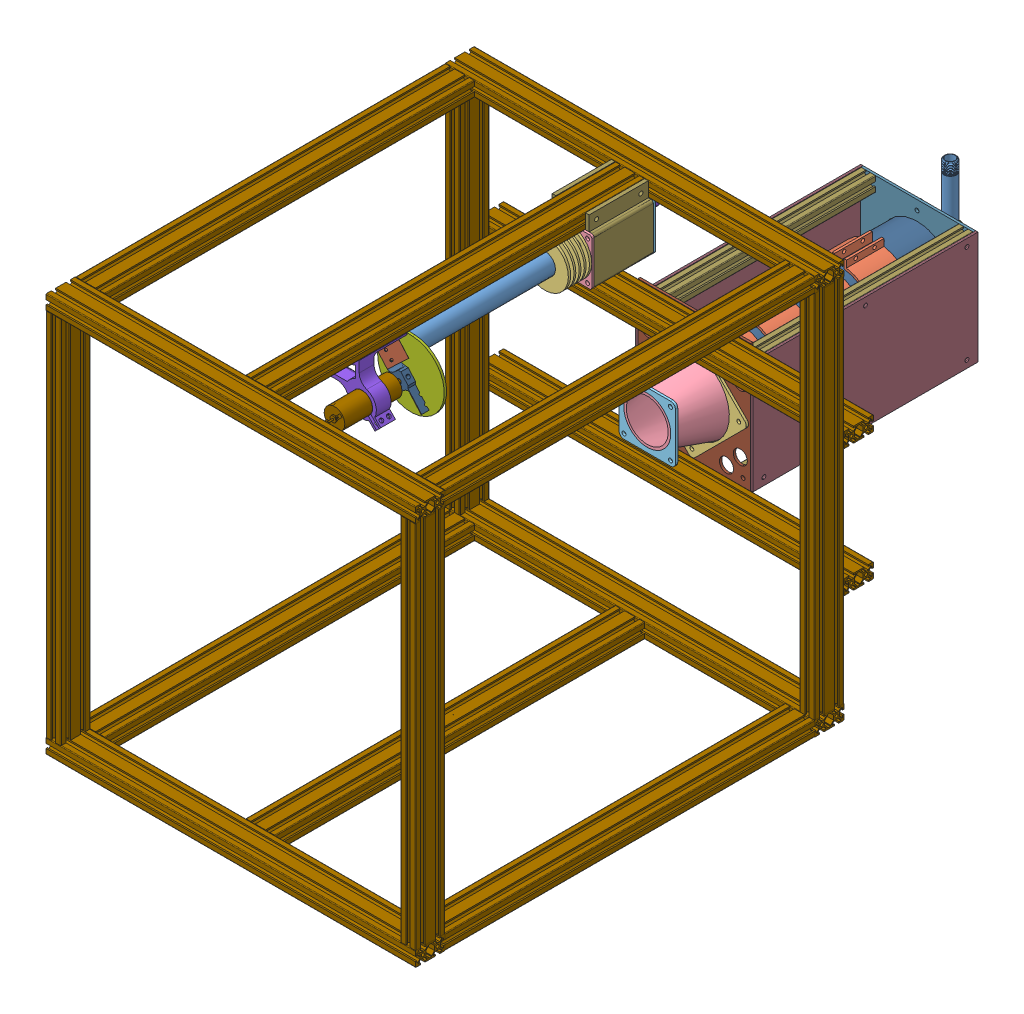
SolidWorks assembly extruder 1 assembly, configuration Default. Lengths in mm.
Overall size (500 540 979.81).
58 component instances, 30 part files, 85 mates.
Components (placement in the parent):
- extruder barrel_rev01-1: extruder barrel_rev01 [Default] at (188.8223 217.5446 43.8354) size (28.57 28.57 304.8)
- nozzle_rev01-1: nozzle_rev01 [Default] at (188.8223 217.5446 329.5854) size (28.57 28.57 31.75)
- barrel lock-1: barrel lock [Default] at (188.8223 217.5446 154.9604) x (-0.997738 -0.067218 0) z (0.067218 -0.997738 0) size (63.5 31.75 63.5)
- barrel lock mount-1: barrel lock mount [Default] at (188.8223 217.5446 120.0354) x (1 0 0) z (0 -1 0) size (63.5 3.17 63.5)
- thrust bearing plate-1: thrust bearing plate [Default] at (188.8223 217.5446 40.0354) x (1 0 0) z (0 1 0) size (63.5 3.17 63.5)
- 5909K310_THRUST NEEDLE-ROLLER BEARING-1: 5909K310_THRUST NEEDLE-ROLLER BEARING [5909K31] at (188.8223 217.5446 42.0304) x (1 0 0) z (0 -1 0) size (23.81 19.84 23.81)
- 5909K440_THRUST NEEDLE-ROLLER BEARING-1: 5909K440_THRUST NEEDLE-ROLLER BEARING [5909K44] at (188.8223 217.5446 41.0382) x (0 0 -1) z (0.082579 0.996584 0) size (0.81 23.81 23.81)
- 5909K440_THRUST NEEDLE-ROLLER BEARING-2: 5909K440_THRUST NEEDLE-ROLLER BEARING [5909K44] at (188.8223 217.5446 43.8354) x (0 0 -1) z (1 0 0) size (0.81 23.81 23.81)
- screw standin-1: screw standin [Default] at (188.8223 217.5446 310.5354) x (1 0 0) z (0 1 0) size (19.55 342.9 19.55)
- 500mm 2040-1: 500mm 2040 [Default] at (188.8223 259.2946 540.0354) x (0 -1 0) z (0 0 1) size (20 40 500)
- 500mm 2040-2: 500mm 2040 [Default] at (-61.3618 259.2946 560.0354) x (0 1 0) z (-1 0 0) size (20 40 500)
- 500mm 2040-3: 500mm 2040 [Default] at (-51.3618 249.2946 560.0354) x (1 0 0) z (0 1 0) size (20 40 500)
- 500mm 2040-4: 500mm 2040 [Default] at (428.6382 -250.7054 560.0354) x (1 0 0) z (0 -1 0) size (20 40 500)
- 500mm 2040-5: 500mm 2040 [Default] at (-61.3618 -260.7054 560.0354) x (0 1 0) z (-1 0 0) size (20 40 500)
- 500mm 2040-6: 500mm 2040 [Default] at (418.6382 259.2946 540.0354) x (0 1 0) z (0 0 1) size (20 40 500)
- 500mm 2040-7: 500mm 2040 [Default] at (-41.3618 259.2946 540.0354) x (0 1 0) z (0 0 1) size (20 40 500)
- 500mm 2040-8: 500mm 2040 [Default] at (418.6382 -260.7054 540.0354) x (0 1 0) z (0 0 1) size (20 40 500)
- 500mm 2040-9: 500mm 2040 [Default] at (-41.3618 -260.7054 540.0354) x (0 -1 0) z (0 0 1) size (20 40 500)
- 500mm 2040-10: 500mm 2040 [Default] at (-61.3618 -260.7054 20.0354) x (0 1 0) z (-1 0 0) size (20 40 500)
- 500mm 2040-11: 500mm 2040 [Default] at (-61.3618 259.2946 20.0354) x (0 -1 0) z (-1 0 0) size (20 40 500)
- 500mm 2040-12: 500mm 2040 [Default] at (-51.3618 249.2946 20.0354) x (-1 0 0) z (0 1 0) size (20 40 500)
- 500mm 2040-13: 500mm 2040 [Default] at (428.6382 249.2946 20.0354) x (1 0 0) z (0 1 0) size (20 40 500)
- 500mm 2040-14: 500mm 2040 [Default] at (188.8164 -260.7054 540.0354) x (0 -1 0) z (0 0 1) size (20 40 500)
- dryer stand alone-1: dryer stand alone [Default] at (381.6192 -132.2091 21.3365) x (0 1 0) z (-1 0 0) size (209.74 423.31 158.7)
  - tube-1: tube [Default] at (103.5422 61.3012 185.6839) size (164.34 304.8 101.6)
  - flange rev01-1: flange rev01 [Default] at (103.5422 61.3012 185.6839) x (-1 0 0) z (0 0 -1) size (192.4 3.17 152.4)
  - HFS5-2020-299-1: HFS5-2020-299 [Default] at (169.7422 63.9262 119.4839) x (-1 0 0) z (0 -1 0) size (20 20 298.45)
  - HFS5-2020-299-2: HFS5-2020-299 [Default] at (37.3422 63.9262 119.4839) x (-1 0 0) z (0 -1 0) size (20 20 298.45)
  - HFS5-2020-299-3: HFS5-2020-299 [Default] at (169.7422 63.9262 251.8839) x (-1 0 0) z (0 -1 0) size (20 20 298.45)
  - HFS5-2020-299-4: HFS5-2020-299 [Default] at (37.3422 363.4762 251.8839) x (-1 0 0) z (0 1 0) size (20 20 298.45)
  - side plate 1_16-1: side plate 1_16 [Default] at (103.5422 213.7012 263.4587) x (-1 0 0) z (0 0 -1) size (152.4 304.8 1.57)
  - side plate 1_16-2: side plate 1_16 [Default] at (103.5422 213.7012 265.0335) x (-1 0 0) z (0 0 -1) size (152.4 304.8 1.57)
  - flange rev02-1: flange rev02 [Default] at (103.5422 362.9262 185.6839) x (-1 0 0) z (0 0 -1) size (152.4 3.17 152.4)
  - top cover-1: top cover [Default] at (103.5422 369.2762 185.6839) x (-0.707107 0 -0.707107) z (0 -1 0) size (107.76 107.76 3.17)
  - 4452K413_TYPE 316 STAINLESS STL THREADED PIPE FITTING-2: 4452K413_TYPE 316 STAINLESS STL THREADED PIPE FITTING [4452K413] at (103.5422 407.8982 185.6839) x (-1 0 0) z (0 0 1) size (37.28 37.03 30.11)
  - 4548K159_STD-WALL TYPE 316-316L SS THRD PIPE NIPPLE-1: 4548K159_STD-WALL TYPE 316-316L SS THRD PIPE NIPPLE [4548K159] at (103.5422 292.6762 185.6839) x (0 1 0) z (0 0 1) size (203.35 17.91 17.78)
  - 4464K498_TYPE 304 STAINLESS STL THREADED PIPE FITTING-1: 4464K498_TYPE 304 STAINLESS STL THREADED PIPE FITTING [4464K498] at (103.5422 180.2482 185.6839) x (-0.837169 0 -0.546944) z (0 1 0) size (25.91 25.91 21.03)
  - 4548K145_STD-WALL TYPE 316-316L SS THRD PIPE NIPPLE-2: 4548K145_STD-WALL TYPE 316-316L SS THRD PIPE NIPPLE [4548K145] at (161.6142 407.8982 185.6839) x (1 0 0) z (0 -0.851872 -0.523749) size (89.04 17.99 18.06)
  - heater band-1: heater band [Default] at (103.5422 257.8762 185.6839) size (116.47 50.8 107.95)
  - heater band-2: heater band [Default] at (103.5422 132.2762 185.6839) size (116.47 50.8 107.95)
  - heater band-3: heater band [Default] at (103.5422 69.4762 185.6839) size (116.47 50.8 107.95)
  - heater band-4: heater band [Default] at (103.5422 195.0762 185.6839) size (116.47 50.8 107.95)
  - bottom cover-1: bottom cover [Default] at (103.6306 61.3012 185.6839) x (-0.707107 0 -0.707107) z (0 -1 0) size (107.76 107.76 3.17)
  - nozzle reduction-1: nozzle reduction [Default] at (103.6306 61.3012 185.6839) x (-0.837169 0 -0.546944) z (-0.546944 0 0.837169) size (101.6 63.5 101.6)
  - 2.5 in bracket-1: 2.5 in bracket [Default] at (103.6306 -2.1988 185.6839) size (76.2 3.17 76.2)
  - side plate 1_16-7: side plate 1_16 [Default] at (103.5422 213.7012 107.9091) size (152.4 304.8 1.57)
  - side plate 1_16-8: side plate 1_16 [Default] at (103.5422 213.7012 106.3343) size (152.4 304.8 1.57)
  - 9157K150_STD-WALL 304-304L SS THRD ONE END PIPE NIPPLE-1: 9157K150_STD-WALL 304-304L SS THRD ONE END PIPE NIPPLE [9157K15] at (103.5422 378.8012 152.0289) x (0 1 0) z (-0.332767 0 0.943009) size (25.49 27.89 27.84)
  - 9157K150_STD-WALL 304-304L SS THRD ONE END PIPE NIPPLE-2: 9157K150_STD-WALL 304-304L SS THRD ONE END PIPE NIPPLE [9157K15] at (103.5422 378.8012 219.3389) x (0 1 0) z (-0.546944 0 0.837169) size (25.49 27.89 27.84)
- pelletizer plate-1: pelletizer plate [Default] at (188.8223 217.5446 361.3354) x (-1 0 0) z (0 -1 0) size (90.17 3.17 90.52)
- pelletizer plate mount-1: pelletizer plate mount [Default] at (188.8223 244.2946 361.3354) x (1 0 0) z (0 -1 0) size (90.17 65 92.21)
- 3262_1-2: 3262_1 [Default] at (212.9094 202.1712 463.8354) x (-0.751023 -0.660276 0) z (0 0 -1) size (28 28 106.2)
- blade wheel-1: blade wheel [Default] at (212.9094 202.1712 366.6354) x (-0.660276 0.751023 0) z (0.751023 0.660276 0) size (76.2 10 20)
- blade fin-1: blade fin [Default] at (228.9848 180.9524 369.3692) x (0.575317 0.505801 0.642788) z (-0.660276 0.751023 0) size (23.8 0.5 23.1)
- blade fin-2: blade fin [Default] at (196.5931 223.1774 368.9862) x (-0.575317 -0.505801 0.642788) z (-0.660276 0.751023 0) size (23.8 0.5 23.1)
- hopper rev02-2: hopper rev02 [Default] at (188.8223 217.5446 120.0354) x (1 0 0) z (0 1 0) size (63.5 80 83.5)
- 500mm 2040-16: 500mm 2040 [Default] at (-61.3618 57.5332 -19.9646) x (0 -1 0) z (-1 0 0) size (20 40 500)
- 500mm 2040-17: 500mm 2040 [Default] at (438.6382 -114.8668 -19.9646) x (0 -1 0) z (1 0 0) size (20 40 500)
Mates (geometry in assembly coordinates):
- Concentric1: concentric anti-aligned: cylinder of extruder barrel_rev01-1 through (188.8223 217.5446 329.5854) axis (0 0 1) radius 11.1125; cylinder of nozzle_rev01-1 through (188.8223 217.5446 348.6354) axis (0 0 -1) radius 11.1125
- Coincident1: coincident anti-aligned: plane of extruder barrel_rev01-1 through (188.8223 217.5446 348.6354) normal (0 0 1); plane of nozzle_rev01-1 through (188.8223 217.5446 348.6354) normal (0 0 -1)
- Concentric2: concentric anti-aligned: cylinder of extruder barrel_rev01-1 through (188.8223 217.5446 348.6354) axis (0 0 -1) radius 14.2875; cylinder of barrel lock-1 through (188.8223 217.5446 123.2104) axis (0 0 1) radius 14.3129
- Distance1: distance = 3.175 mm aligned: plane of barrel lock-1 through (188.8223 217.5446 123.2104) normal (0 0 -1); plane of extruder barrel_rev01-1 through (188.8223 217.5446 120.0354) normal (0 0 -1)
- Concentric3: concentric anti-aligned: cylinder of extruder barrel_rev01-1 through (188.8223 217.5446 348.6354) axis (0 0 -1) radius 14.2875; cylinder of barrel lock mount-1 through (188.8223 217.5446 120.0344) axis (0 0 1) radius 14.3129
- Coincident5: coincident anti-aligned: plane of barrel lock-1 through (188.8223 217.5446 123.2104) normal (0 0 -1); plane of barrel lock mount-1 through (188.8223 217.5446 123.2104) normal (0 0 1)
- Concentric4: concentric anti-aligned: cylinder of extruder barrel_rev01-1 through (188.8223 217.5446 348.6354) axis (0 0 -1) radius 9.525; cylinder of 5909K440_THRUST NEEDLE-ROLLER BEARING-2 through (188.8223 217.5446 43.0226) axis (0 0 1) radius 6.3754
- Concentric5: concentric anti-aligned: cylinder of 5909K310_THRUST NEEDLE-ROLLER BEARING-1 through (188.8223 217.5446 41.0382) axis (0 0 -1) radius 6.3754; cylinder of 5909K440_THRUST NEEDLE-ROLLER BEARING-2 through (188.8223 217.5446 43.0226) axis (0 0 1) radius 6.3754
- Tangent1: tangent anti-aligned: cylinder of 5909K310_THRUST NEEDLE-ROLLER BEARING-1 through (195.7165 208.687 42.0304) axis (0.614213 -0.789141 0) radius 0.9922; plane of 5909K440_THRUST NEEDLE-ROLLER BEARING-2 through (188.8223 217.5446 43.0226) normal (0 0 -1)
- Concentric7: concentric anti-aligned: cylinder of 5909K310_THRUST NEEDLE-ROLLER BEARING-1 through (188.8223 217.5446 41.0382) axis (0 0 -1) radius 6.3754; cylinder of 5909K440_THRUST NEEDLE-ROLLER BEARING-1 through (188.8223 217.5446 40.2254) axis (0 0 1) radius 6.3754
- Tangent3: tangent anti-aligned: cylinder of 5909K310_THRUST NEEDLE-ROLLER BEARING-1 through (179.4256 211.4054 42.0304) axis (-0.837166 -0.546948 0) radius 0.9922; plane of 5909K440_THRUST NEEDLE-ROLLER BEARING-1 through (188.8223 217.5446 41.0382) normal (0 0 1)
- Concentric8: concentric anti-aligned: cylinder of extruder barrel_rev01-1 through (188.8223 217.5446 348.6354) axis (0 0 -1) radius 9.525; cylinder of screw standin-1 through (188.8223 217.5446 43.8354) axis (0 0 1) radius 9.525
- Coincident17: coincident anti-aligned: plane of 5909K440_THRUST NEEDLE-ROLLER BEARING-2 through (188.8223 217.5446 43.8354) normal (0 0 1); plane of screw standin-1 through (188.8223 217.5446 43.8354) normal (0 0 -1)
- Coincident18: coincident aligned: plane of barrel lock mount-1 through (220.5723 249.2946 123.2104) normal (0 1 0); plane of thrust bearing plate-1 through (157.0723 249.2946 36.8604) normal (0 1 0)
- Coincident19: coincident aligned: plane of barrel lock mount-1 through (157.0723 185.7946 123.2104) normal (-1 0 0); plane of thrust bearing plate-1 through (157.0723 249.2946 36.8604) normal (-1 0 0)
- Distance2: distance = 80 mm anti-aligned: plane of thrust bearing plate-1 through (188.8223 217.5446 40.0354) normal (0 0 1); plane of barrel lock mount-1 through (188.8223 217.5446 120.0354) normal (0 0 -1)
- Coincident32: coincident aligned: plane of 500mm 2040-1 through (195.8223 269.2946 40.0354) normal (0 1 0); plane of 500mm 2040-2 through (438.6382 269.2946 567.0354) normal (0 1 0)
- Coincident33: coincident anti-aligned: plane of 500mm 2040-1 through (169.8223 268.2946 540.0354) normal (0 0 1); plane of 500mm 2040-2 through (438.6382 256.2946 540.0354) normal (0 0 -1)
- Coincident34: coincident anti-aligned: plane of 500mm 2040-2 through (438.6382 249.2946 553.0354) normal (0 -1 0); plane of 500mm 2040-3 through (-60.3618 249.2946 579.0354) normal (0 1 0)
- Coincident35: coincident aligned: plane of 500mm 2040-2 through (-61.3618 250.2946 579.0354) normal (-1 0 0); plane of 500mm 2040-3 through (-61.3618 -250.7054 553.0354) normal (-1 0 0)
- Coincident36: coincident aligned: plane of 500mm 2040-2 through (438.6382 256.2946 540.0354) normal (0 0 -1); plane of 500mm 2040-3 through (-54.3618 -250.7054 540.0354) normal (0 0 -1)
- Coincident37: coincident anti-aligned: plane of 500mm 2040-2 through (438.6382 249.2946 553.0354) normal (0 -1 0); plane of 500mm 2040-4 through (419.6382 249.2946 541.0354) normal (0 1 0)
- Coincident38: coincident aligned: plane of 500mm 2040-2 through (438.6382 256.2946 540.0354) normal (0 0 -1); plane of 500mm 2040-4 through (431.6382 249.2946 540.0354) normal (0 0 -1)
- Coincident39: coincident aligned: plane of 500mm 2040-2 through (438.6382 250.2946 579.0354) normal (1 0 0); plane of 500mm 2040-4 through (438.6382 249.2946 541.0354) normal (1 0 0)
- Coincident40: coincident anti-aligned: plane of 500mm 2040-3 through (-60.3618 -250.7054 579.0354) normal (0 -1 0); plane of 500mm 2040-5 through (438.6382 -250.7054 567.0354) normal (0 1 0)
- Coincident41: coincident aligned: plane of 500mm 2040-4 through (437.6382 249.2946 580.0354) normal (0 0 1); plane of 500mm 2040-5 through (438.6382 -257.7054 580.0354) normal (0 0 1)
- Coincident42: coincident aligned: plane of 500mm 2040-4 through (438.6382 249.2946 541.0354) normal (1 0 0); plane of 500mm 2040-5 through (438.6382 -269.7054 579.0354) normal (1 0 0)
- Coincident43: coincident anti-aligned: plane of 500mm 2040-2 through (438.6382 256.2946 540.0354) normal (0 0 -1); plane of 500mm 2040-6 through (437.6382 250.2946 540.0354) normal (0 0 1)
- Coincident44: coincident aligned: plane of 500mm 2040-2 through (438.6382 269.2946 567.0354) normal (0 1 0); plane of 500mm 2040-6 through (425.6382 269.2946 40.0354) normal (0 1 0)
- Coincident45: coincident aligned: plane of 500mm 2040-2 through (438.6382 250.2946 579.0354) normal (1 0 0); plane of 500mm 2040-6 through (438.6382 262.2946 40.0354) normal (1 0 0)
- Coincident46: coincident anti-aligned: plane of 500mm 2040-2 through (438.6382 256.2946 540.0354) normal (0 0 -1); plane of 500mm 2040-7 through (-22.3618 250.2946 540.0354) normal (0 0 1)
- Coincident47: coincident aligned: plane of 500mm 2040-2 through (-61.3618 250.2946 579.0354) normal (-1 0 0); plane of 500mm 2040-7 through (-61.3618 268.2946 40.0354) normal (-1 0 0)
- Coincident48: coincident aligned: plane of 500mm 2040-2 through (438.6382 269.2946 547.0354) normal (0 1 0); plane of 500mm 2040-7 through (-34.3618 269.2946 40.0354) normal (0 1 0)
- Coincident49: coincident anti-aligned: plane of 500mm 2040-5 through (438.6382 -251.7054 540.0354) normal (0 0 -1); plane of 500mm 2040-8 through (437.6382 -269.7054 540.0354) normal (0 0 1)
- Coincident50: coincident aligned: plane of 500mm 2040-5 through (438.6382 -269.7054 579.0354) normal (1 0 0); plane of 500mm 2040-8 through (438.6382 -257.7054 40.0354) normal (1 0 0)
- Coincident51: coincident aligned: plane of 500mm 2040-5 through (438.6382 -270.7054 541.0354) normal (0 -1 0); plane of 500mm 2040-8 through (411.6382 -270.7054 40.0354) normal (0 -1 0)
- Coincident52: coincident anti-aligned: plane of 500mm 2040-5 through (438.6382 -251.7054 540.0354) normal (0 0 -1); plane of 500mm 2040-9 through (-60.3618 -251.7054 540.0354) normal (0 0 1)
- Coincident53: coincident aligned: plane of 500mm 2040-5 through (-61.3618 -269.7054 579.0354) normal (-1 0 0); plane of 500mm 2040-9 through (-61.3618 -251.7054 40.0354) normal (-1 0 0)
- Coincident54: coincident aligned: plane of 500mm 2040-5 through (438.6382 -270.7054 541.0354) normal (0 -1 0); plane of 500mm 2040-9 through (-60.3618 -270.7054 40.0354) normal (0 -1 0)
- Coincident55: coincident anti-aligned: plane of 500mm 2040-8 through (437.6382 -269.7054 40.0354) normal (0 0 -1); plane of 500mm 2040-10 through (438.6382 -269.7054 40.0354) normal (0 0 1)
- Coincident56: coincident aligned: plane of 500mm 2040-8 through (438.6382 -257.7054 40.0354) normal (1 0 0); plane of 500mm 2040-10 through (438.6382 -269.7054 39.0354) normal (1 0 0)
- Coincident57: coincident aligned: plane of 500mm 2040-8 through (411.6382 -270.7054 40.0354) normal (0 -1 0); plane of 500mm 2040-10 through (438.6382 -270.7054 33.0354) normal (0 -1 0)
- Coincident58: coincident anti-aligned: plane of 500mm 2040-6 through (437.6382 250.2946 40.0354) normal (0 0 -1); plane of 500mm 2040-11 through (438.6382 262.2946 40.0354) normal (0 0 1)
- Coincident59: coincident aligned: plane of 500mm 2040-6 through (438.6382 262.2946 40.0354) normal (1 0 0); plane of 500mm 2040-11 through (438.6382 268.2946 1.0354) normal (1 0 0)
- Coincident60: coincident aligned: plane of 500mm 2040-6 through (425.6382 269.2946 40.0354) normal (0 1 0); plane of 500mm 2040-11 through (438.6382 269.2946 39.0354) normal (0 1 0)
- Coincident61: coincident aligned: plane of 500mm 2040-7 through (-34.3618 269.2946 40.0354) normal (0 1 0); plane of 500mm 2040-11 through (438.6382 269.2946 27.0354) normal (0 1 0)
- Coincident62: coincident aligned: plane of 500mm 2040-11 through (438.6382 256.2946 0.0354) normal (0 0 -1); plane of 500mm 2040-12 through (-42.3618 -250.7054 0.0354) normal (0 0 -1)
- Coincident63: coincident anti-aligned: plane of 500mm 2040-10 through (438.6382 -250.7054 27.0354) normal (0 1 0); plane of 500mm 2040-12 through (-42.3618 -250.7054 1.0354) normal (0 -1 0)
- Coincident64: coincident aligned: plane of 500mm 2040-10 through (-61.3618 -269.7054 39.0354) normal (-1 0 0); plane of 500mm 2040-12 through (-61.3618 -250.7054 13.0354) normal (-1 0 0)
- Coincident65: coincident aligned: plane of 500mm 2040-11 through (-61.3618 268.2946 1.0354) normal (-1 0 0); plane of 500mm 2040-12 through (-61.3618 -250.7054 13.0354) normal (-1 0 0)
- Coincident66: coincident anti-aligned: plane of 500mm 2040-10 through (438.6382 -250.7054 27.0354) normal (0 1 0); plane of 500mm 2040-13 through (419.6382 -250.7054 39.0354) normal (0 -1 0)
- Coincident67: coincident aligned: plane of 500mm 2040-10 through (438.6382 -269.7054 39.0354) normal (1 0 0); plane of 500mm 2040-13 through (438.6382 -250.7054 27.0354) normal (1 0 0)
- Coincident68: coincident aligned: plane of 500mm 2040-10 through (438.6382 -251.7054 0.0354) normal (0 0 -1); plane of 500mm 2040-13 through (437.6382 -250.7054 0.0354) normal (0 0 -1)
- Coincident69: coincident anti-aligned: plane of 500mm 2040-5 through (438.6382 -251.7054 540.0354) normal (0 0 -1); plane of 500mm 2040-14 through (169.8164 -251.7054 540.0354) normal (0 0 1)
- Coincident70: coincident aligned: plane of 500mm 2040-5 through (438.6382 -270.7054 553.0354) normal (0 -1 0); plane of 500mm 2040-14 through (181.8164 -270.7054 40.0354) normal (0 -1 0)
- Parallel4: parallel anti-aligned: plane of 500mm 2040-11 through (438.6382 256.2946 0.0354) normal (0 0 -1); plane of dryer stand alone-1/2.5 in bracket-1 through (195.9354 -28.5784 23.5354) normal (0 0 1)
- Coincident89: coincident aligned: plane of nozzle_rev01-1 through (188.8223 217.5446 361.3354) normal (0 0 1); plane of pelletizer plate-1 through (188.8223 217.5446 361.3354) normal (0 0 1)
- Coincident90: coincident anti-aligned: plane of 500mm 2040-1 through (181.8223 249.2946 40.0354) normal (0 -1 0); plane of pelletizer plate-1 through (188.8223 249.2946 358.1604) normal (0 1 0)
- Concentric9: concentric anti-aligned: cylinder of nozzle_rev01-1 through (188.8223 217.5446 361.3354) axis (0 0 -1) radius 14.2875; cylinder of pelletizer plate-1 through (188.8223 217.5446 358.1604) axis (0 0 1) radius 13.335
- Coincident91: coincident anti-aligned: plane of 500mm 2040-1 through (181.8223 249.2946 40.0354) normal (0 -1 0); plane of pelletizer plate mount-1 through (168.8223 249.2946 426.3354) normal (0 1 0)
- Coincident92: coincident anti-aligned: plane of pelletizer plate-1 through (188.8223 217.5446 361.3354) normal (0 0 1); plane of pelletizer plate mount-1 through (188.8223 244.2946 361.3354) normal (0 0 -1)
- Coincident93: coincident aligned: plane of 500mm 2040-1 through (168.8223 256.2946 40.0354) normal (-1 0 0); plane of pelletizer plate mount-1 through (168.8223 239.2946 426.3354) normal (-1 0 0)
- Concentric12: concentric aligned: cylinder of 3262_1-2 through (212.9094 202.1712 383.3354) axis (0 0 -1) radius 3; cylinder of blade wheel-1 through (212.9094 202.1712 376.6354) axis (0 0 -1) radius 3.165
- Parallel7: parallel aligned: plane of 3262_1-2 through (214.795 203.829 381.3354) normal (0.751023 0.660276 0); plane of blade wheel-1 through (227.0224 201.2638 338.3511) normal (0.751023 0.660276 0)
- Parallel8: parallel anti-aligned: plane of 3262_1-2 through (212.9094 202.1712 384.3354) normal (0 0 -1); plane of blade wheel-1 through (212.9094 202.1712 376.6354) normal (0 0 1)
- Coincident96: coincident aligned: plane of 3262_1-2 through (213.03 202.2772 366.6354) normal (0 0 -1); plane of blade wheel-1 through (212.9094 202.1712 366.6354) normal (0 0 -1)
- Distance3: distance = 20 mm aligned: plane of 3262_1-2 through (212.9094 202.1712 386.3354) normal (0 0 -1); plane of pelletizer plate mount-1 through (212.9094 202.1712 406.3354) normal (0 0 -1)
- Coincident100: coincident anti-aligned: plane of blade wheel-1 through (225.1448 199.6131 376.6354) normal (-0.482748 -0.424417 0.766044); plane of blade fin-1 through (229.2261 181.1646 368.9862) normal (0.482748 0.424417 -0.766044)
- Coincident101: coincident aligned: plane of blade wheel-1 through (243.6986 178.5093 376.6354) normal (0.660276 -0.751023 0); plane of blade fin-1 through (230.0061 166.4713 361.337) normal (0.660276 -0.751023 0)
- Coincident102: coincident: line of blade wheel-1 through (243.6986 178.5093 376.6354) axis (-0.660276 0.751023 0); plane of blade fin-1 through (243.6986 178.5093 376.6354) normal (0.575317 0.505801 0.642788)
- Coincident103: coincident anti-aligned: plane of blade wheel-1 through (200.674 204.7294 376.6354) normal (0.482748 0.424417 0.766044); plane of blade fin-2 through (196.5931 223.1774 368.9862) normal (-0.482748 -0.424417 -0.766044)
- Concentric13: concentric aligned: cylinder of blade wheel-1 through (186.083 221.3271 364.5351) axis (0.482748 0.424417 0.766044) radius 2.5; cylinder of blade fin-2 through (190.557 225.2605 371.6346) axis (0.482748 0.424417 0.766044) radius 1.665
- Concentric14: concentric aligned: cylinder of blade wheel-1 through (193.4116 212.9912 364.5351) axis (0.482748 0.424417 0.766044) radius 2.5; cylinder of blade fin-2 through (197.8856 216.9247 371.6346) axis (0.482748 0.424417 0.766044) radius 1.665
- Coincident104: coincident anti-aligned: plane of barrel lock mount-1 through (188.8223 217.5446 120.0354) normal (0 0 -1); plane of hopper rev02-2 through (188.8223 217.5446 120.0354) normal (0 0 1)
- Coincident105: coincident aligned: plane of barrel lock mount-1 through (220.5723 185.7946 123.2104) normal (1 0 0); plane of hopper rev02-2 through (220.5723 185.7946 40.0354) normal (1 0 0)
- Coincident106: coincident aligned: plane of barrel lock mount-1 through (220.5723 185.7946 123.2104) normal (0 -1 0); plane of hopper rev02-2 through (157.0723 185.7946 40.0354) normal (0 -1 0)
- Coincident114: coincident anti-aligned: plane of 500mm 2040-13 through (437.6382 -250.7054 0.0354) normal (0 0 -1); plane of 500mm 2040-16 through (438.6382 48.5332 0.0354) normal (0 0 1)
- Coincident116: coincident aligned: plane of 500mm 2040-13 through (438.6382 -250.7054 27.0354) normal (1 0 0); plane of 500mm 2040-16 through (438.6382 66.5332 -38.9646) normal (1 0 0)
- Coincident117: coincident anti-aligned: plane of dryer stand alone-1/flange rev01-1 through (195.9354 -28.6668 -39.9646) normal (0 0 1); plane of 500mm 2040-16 through (438.6382 54.5332 -39.9646) normal (0 0 -1)
- Coincident118: coincident aligned: plane of dryer stand alone-1/flange rev01-1 through (195.9354 67.5332 -39.9646) normal (0 1 0); plane of 500mm 2040-16 through (438.6382 67.5332 -32.9646) normal (0 1 0)
- Coincident119: coincident anti-aligned: plane of 500mm 2040-1 through (208.8223 262.2946 40.0354) normal (1 0 0); plane of hopper rev02-2 through (208.8223 269.2946 40.0354) normal (-1 0 0)
- Coincident120: coincident anti-aligned: plane of 500mm 2040-12 through (-42.3618 -250.7054 0.0354) normal (0 0 -1); plane of 500mm 2040-17 through (-61.3618 -117.8668 0.0354) normal (0 0 1)
- Coincident121: coincident aligned: plane of 500mm 2040-12 through (-61.3618 -250.7054 13.0354) normal (-1 0 0); plane of 500mm 2040-17 through (-61.3618 -105.8668 -0.9646) normal (-1 0 0)
- Coincident122: coincident aligned: plane of dryer stand alone-1/flange rev01-1 through (195.9354 -124.8668 -39.9646) normal (0 -1 0); plane of 500mm 2040-17 through (-61.3618 -124.8668 -12.9646) normal (0 -1 0)
- Coincident123: coincident anti-aligned: plane of 500mm 2040-11 through (438.6382 262.2946 40.0354) normal (0 0 1); plane of hopper rev02-2 through (188.8223 217.5446 40.0354) normal (0 0 -1)
